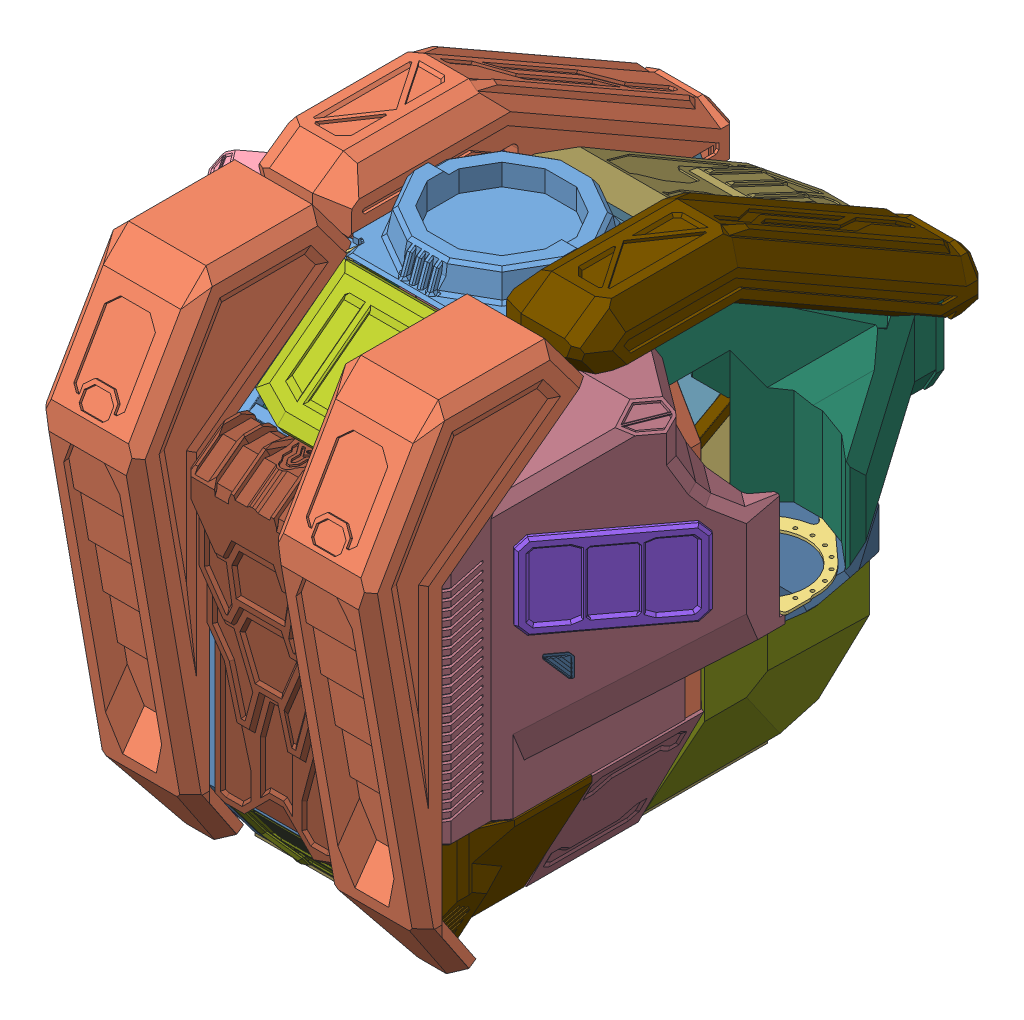
SolidWorks assembly cockpite superficie, configuration Défaut. Lengths in mm. (continued)
Mates (geometry in assembly coordinates): (continued)
- Coaxiale6: concentric anti-aligned: cylinder of axeO20.25_700-1 through (100 1702.1061 -146.8375) axis (-1 0 0) radius 10; cylinder of Capot-1/Capot1-1 through (-490 1702.1061 -146.8375) axis (1 0 0) radius 10
- Distance5: distance = 10 mm anti-aligned: plane of Capot-1/Capot1-1 through (-490 1702.1061 -146.8375) normal (-1 0 0); plane of cockpit_segmentLAT_0-2 through (-500 0 0) normal (1 0 0)
- Coïncidente146: coincident anti-aligned: plane of bras_fixation_1-2 through (-1040 990 -47.0887) normal (0 -1 0); plane of deco_torse2LEFT-1 through (-931.6884 990 -630) normal (0 1 0)
- Coïncidente147: coincident anti-aligned: plane of cockpit_segmentLAT_0-2 through (-500 0 -740) normal (0 0 -1); plane of deco_torse2LEFT-1 through (-173.0822 150 -740) normal (0 0 1)
- Coïncidente148: coincident anti-aligned: plane of cockpit_segmentLAT_0-1 through (80 0 -740) normal (0 0 -1); plane of deco_torse2RIGHT-1 through (336.2329 150 -740) normal (0 0 1)
- Coïncidente149: coincident anti-aligned: plane of bras_fixation_1-1 through (540 990 -47.0887) normal (0 -1 0); plane of deco_torse2RIGHT-1 through (431.6884 990 -630) normal (0 1 0)
- Coïncidente150: coincident anti-aligned: plane of cockpit_segment_40x40_0-3 through (338 1000 -10) normal (0.942847 0 -0.333225); plane of deco_torse2RIGHT-1 through (336.2329 1000 -15) normal (-0.942847 0 0.333225)
- Coïncidente152: coincident anti-aligned: plane of cockpit_segment_40x40_0-4 through (-838 960 -10) normal (-0.942847 0 -0.333225); plane of deco_torse2LEFT-1 through (-836.2329 1000 -15) normal (0.942847 0 0.333225)
- Coïncidente153: coincident anti-aligned: plane of bras_fixation_1-1 through (540 1000 -47.0887) normal (0 1 0); plane of deco_torse1-1 through (277.9178 1000 -180) normal (0 -1 0)
- Coïncidente156: coincident anti-aligned: plane of cockpit_segmentLAT_0-1 through (80 0 -740) normal (0 0 -1); plane of deco_torse1-1 through (277.9178 1000 -740) normal (0 0 1)
- Coïncidente157: coincident anti-aligned: plane of cockpit_segment_40x40_0-1 through (338 1323.2129 -10) normal (0.942847 0 -0.333225); plane of deco_torse1-1 through (277.9178 1350 -180) normal (-0.942847 0 0.333225)
- Coïncidente166: coincident anti-aligned: plane of cockpit_segmentFACE_0-2 through (-593.1411 1740 413.3333) normal (0 1 0); plane of deco_headcollar-1 through (-540 1740 423.19) normal (0 -1 0)
- Coïncidente171: coincident anti-aligned: plane of cockpit_segmentLAT_0-1 through (80 1312 984) normal (0 0.8 0.6); plane of deco_torse4_back-1/deco_torse4_back-1 through (370 1630 560) normal (0 -0.8 -0.6)
- Coïncidente172: coincident anti-aligned: plane of cockpit_segmentLAT_0-2 through (-500 1312 984) normal (0 0.8 0.6); plane of deco_torse4_back-2/deco_torse4_back-1 through (-500 1630 560) normal (0 -0.8 -0.6)
- Coïncidente174: coincident anti-aligned: plane of cockpit_segmentLAT_0-1 through (80 0 960) normal (0 0 1); plane of deco_torse4_back-1/deco_torse4_back-1 through (370 250 960) normal (0 0 -1)
- Coïncidente175: coincident anti-aligned: plane of cockpit_segmentLAT_0-2 through (-500 0 960) normal (0 0 1); plane of deco_torse4_back-2/deco_torse4_back-1 through (-500 250 960) normal (0 0 -1)
- Coïncidente176: coincident aligned: plane of cockpit_segmentLAT_0-1 through (0 0 0) normal (-1 0 0); plane of attache_porte2-2 through (0 1717.0991 489.9076) normal (-1 0 0)
- Coïncidente177: coincident anti-aligned: plane of cockpit_segmentLAT_0-1 through (80 1312 984) normal (0 0.8 0.6); plane of attache_porte2-2 through (10 1737 417.3333) normal (0 -0.8 -0.6)
- Coïncidente180: coincident anti-aligned: plane of cockpit_segmentLAT_0-2 through (-500 1312 984) normal (0 0.8 0.6); plane of attache_porte2-4 through (-500 1737 417.3333) normal (0 -0.8 -0.6)
- Coïncidente181: coincident aligned: plane of cockpit_segmentLAT_0-2 through (-500 0 0) normal (1 0 0); plane of attache_porte2-4 through (-500 1717.0991 489.9076) normal (1 0 0)
- Coaxiale7: concentric aligned: cylinder of attache_porte2-2 through (10 1717.0991 489.9076) axis (-1 0 0) radius 23.5; cylinder of attache_porte2-4 through (-500 1717.0991 489.9076) axis (-1 0 0) radius 23.5
- Coïncidente182: coincident anti-aligned: plane of cockpit_segment_40x40_2_back-2 through (-840 1310.6802 413.3333) normal (-0.902861 0 0.429934); plane of deco_torse5_back-1 through (-674.9206 450 760) normal (0.902861 0 -0.429934)
- Coïncidente186: coincident aligned: plane of cockpit_segmentLAT_0-2 through (-500 0 0) normal (1 0 0); plane of deco_torse4_back-2/deco_torse4_back-1 through (-500 250 960) normal (1 0 0)
- Coïncidente189: coincident anti-aligned: plane of deco_torse4_back-2/deco_torse4_back-1 through (-500 250 960) normal (0 0 -1); plane of deco_torse5_back-1 through (-824.9206 450 960) normal (0 0 1)
- Coïncidente191: coincident anti-aligned: plane of cockpit_segmentLAT_0-2 through (-500 0 -740) normal (0 0 -1); plane of deco_torse1_sym-1 through (-238.4658 1000 -740) normal (0 0 1)
- Coïncidente194: coincident aligned: plane of deco_torse1-1 through (277.9178 1000 -180) normal (0 -1 0); plane of deco_torse1_sym-1 through (-777.9178 1000 -180) normal (0 -1 0)
- Coïncidente195: coincident anti-aligned: plane of cockpit_segment_40x40_0-2 through (-838 1283.2129 -10) normal (-0.942847 0 -0.333225); plane of deco_torse1_sym-1 through (-777.9178 1350 -180) normal (0.942847 0 0.333225)
- Coïncidente197: coincident: plane of deco_headcollar-1 through (-540 1740 423.19) normal (0 -1 0); line of attache_porte2-4 through (-500 1740 413.3333) axis (-1 0 0)
- Coaxiale8: concentric anti-aligned: cylinder of attache_porte2-2 through (10 1717.0991 489.9076) axis (-1 0 0) radius 23.5; cylinder of axeO20_520-1 through (-510 1717.0991 489.9076) axis (1 0 0) radius 10
- Coïncidente198: coincident aligned: plane of attache_porte2-4 through (-510 1717.0991 489.9076) normal (-1 0 0); plane of axeO20_520-1 through (-510 1717.0991 489.9076) normal (-1 0 0)
- Coaxiale9: concentric anti-aligned: cylinder of axeO20_520-1 through (-510 1717.0991 489.9076) axis (1 0 0) radius 10; cylinder of écoutille1-1 through (-5 1717.0991 489.9076) axis (-1 0 0) radius 10
- Distance8: distance = 5 mm anti-aligned: plane of écoutille1-1 through (-495 1761.0064 498.4018) normal (-1 0 0); plane of cockpit_segmentLAT_0-2 through (-500 0 0) normal (1 0 0)
- Coïncidente200: coincident anti-aligned: plane of deco_torse5_back-1 through (-1147.1119 1368.7153 314.3167) normal (0 -1 0); plane of back_trap-1 through (-1155.1093 1368.7153 320.3201) normal (0 1 0)
- Coïncidente201: coincident anti-aligned: plane of deco_torse5_back-1 through (-1165.1221 1098.7153 290.3244) normal (0.600343 0 0.799743); plane of back_trap-1 through (-1173.1196 1098.7153 296.3278) normal (-0.600343 0 -0.799743)
- Coïncidente202: coincident anti-aligned: plane of deco_torse5_back-1 through (-1234.9206 450 214) normal (-0.799743 0 0.600343); plane of back_trap-1 through (-1173.1196 1068.7153 296.3278) normal (0.799743 0 -0.600343)
- Coïncidente203: coincident anti-aligned: plane of bras_fixation_1-2 through (-1040 990 -47.0887) normal (0 -1 0); plane of deco_torse6_airvent-1 through (-834.9206 990 -640.6226) normal (0 1 0)
- Coïncidente204: coincident aligned: plane of deco_torse5_back-1 through (-1234.9206 450 69) normal (-1 0 0); plane of deco_torse6_airvent-1 through (-1234.9206 958 -640.6226) normal (-1 0 0)
- Coïncidente205: coincident anti-aligned: plane of deco_torse5_back-1 through (-1234.9206 450 214) normal (-0.799743 0 0.600343); plane of airvent-1 through (-958.7971 986.7153 581.836) normal (0.799743 0 -0.600343)
- Coïncidente206: coincident anti-aligned: plane of deco_torse5_back-1 through (-945.997 968.7153 582.2305) normal (0.600343 0 0.799743); plane of airvent-1 through (-949.9957 909.7153 585.2322) normal (-0.600343 0 -0.799743)
- Coïncidente207: coincident anti-aligned: plane of deco_torse5_back-1 through (-939.9935 978.7153 590.2279) normal (0 -1 0); plane of airvent-1 through (-943.8039 978.7153 593.4805) normal (0 1 0)
- Coïncidente208: coincident anti-aligned: plane of cockpit_poutre40x80x500-6 through (-500 1328 960) normal (0 0 1); plane of deco_torse7_dos-1 through (-500 230 960) normal (0 0 -1)
- Coïncidente211: coincident anti-aligned: plane of deco_torse4_back-1/deco_torse4_back-1 through (0 250 960) normal (-1 0 0); plane of deco_torse7_dos-1 through (0 230 960) normal (1 0 0)
- Coïncidente212: coincident anti-aligned: plane of cockpit_segmentLAT_0-1 through (80 1312 984) normal (0 0.8 0.6); plane of deco_torse7_dos-1 through (-500 1330 960) normal (0 -0.8 -0.6)
- Coïncidente213: coincident anti-aligned: plane of cockpit_segmentLAT_0-1 through (80 -40 0) normal (0 -1 0); plane of plancher-1 through (-580 -40 740.5405) normal (0 1 0)
- Coïncidente214: coincident: plane of cockpit_segmentLAT_0-1 through (80 0 0) normal (1 0 0); line of plancher-1 through (80 -40 740.5405) axis (0 0 -1)
- Coïncidente216: coincident: line of cockpit_segmentLAT_0-1 through (78 -40 740.5405) axis (-1 0 0); plane of plancher-1 through (-580 -40 740.5405) normal (0 0 1)
- Coïncidente219: coincident anti-aligned: plane of cockpit_segmentFACE_0-1 through (-840 440.3702 69.3774) normal (-0.890435 -0.455111 0); plane of deco_torse8_lateralinferieur-1 through (-599.1619 -30.8347 -6.6667) normal (0.890435 0.455111 0)
- Coïncidente220: coincident aligned: plane of cockpit_segmentFACE_0-2 through (-250 0 413.3333) normal (0 0 1); plane of deco_torse8_lateralinferieur-1 through (-608.0663 -35.3858 413.3333) normal (0 0 1)
- Coïncidente221: coincident: plane of deco_torse5_back-1 through (-674.9206 450 214) normal (0 -1 0); line of deco_torse8_lateralinferieur-1 through (-844.9219 450 413.3333) axis (0 0 -1)
- Coïncidente224: coincident anti-aligned: plane of cockpit_segmentFACE_0-1 through (340 440.3702 69.3774) normal (0.890435 -0.455111 0); plane of deco_torse8_lateralinferieur-2 through (99.1619 -30.8347 413.3333) normal (-0.890435 0.455111 0)
- Coïncidente225: coincident aligned: plane of cockpit_segmentFACE_0-2 through (-250 0 413.3333) normal (0 0 1); plane of deco_torse8_lateralinferieur-2 through (108.0663 -35.3858 413.3333) normal (0 0 1)
- Coïncidente226: coincident aligned: plane of cockpit_segmentLAT_0-1 through (0 0 0) normal (-1 0 0); plane of attache_porte-5 through (0 32.3991 -638.0132) normal (-1 0 0)
- Coïncidente227: coincident anti-aligned: plane of cockpit_segmentLAT_0-1 through (80 -278.2843 -278.2843) normal (0 -0.707107 -0.707107); plane of attache_porte-5 through (10 -33.8763 -522.6923) normal (0 0.707107 0.707107)
- Coïncidente228: coincident anti-aligned: plane of cockpit_segmentLAT_0-2 through (-500 -278.2843 -278.2843) normal (0 -0.707107 -0.707107); plane of attache_porte-6 through (-500 -33.8763 -522.6923) normal (0 0.707107 0.707107)
- Coïncidente229: coincident aligned: plane of cockpit_segmentLAT_0-2 through (-500 0 0) normal (1 0 0); plane of attache_porte-6 through (-500 32.3991 -638.0132) normal (1 0 0)
- Coïncidente230: coincident aligned: line of attache_porte-5 through (10 -40 -516.5685) axis (-1 0 0); line of attache_porte-6 through (-500 -40 -516.5685) axis (-1 0 0)
- Coïncidente232: coincident: plane of plancher-1 through (-580 -40 740.5405) normal (0 1 0); line of attache_porte-5 through (10 -40 -516.5685) axis (-1 0 0)
- Coïncidente233: coincident aligned: plane of attache_porte-5 through (10 32.3991 -638.0132) normal (1 0 0); plane of axeO20_520-2 through (10 32.3991 -638.0132) normal (1 0 0)
- Coaxiale10: concentric anti-aligned: cylinder of attache_porte-6 through (-500 32.3991 -638.0132) axis (-1 0 0) radius 23.5; cylinder of axeO20_520-2 through (-510 32.3991 -638.0132) axis (1 0 0) radius 10
- Coïncidente237: coincident anti-aligned: plane of cockpit_segmentLAT_0-1 through (80 -59.667 129.9889) normal (0 0.417168 -0.90883); plane of internalpanel1_back-1 through (-580 1402.9178 801.3393) normal (0 -0.417168 0.90883)
- Coïncidente238: coincident aligned: plane of cockpit_segmentLAT_0-2 through (-580 0 0) normal (-1 0 0); plane of internalpanel1_back-1 through (-580 1407.0895 792.251) normal (-1 0 0)
- Coïncidente239: coincident aligned: line of cockpit_segmentLAT_0-2 through (-502 485 380) axis (-1 0 0); line of internalpanel1_back-1 through (80 485 380) axis (-1 0 0)
- Coïncidente240: coincident anti-aligned: plane of cockpit_segmentFACE_0-1 through (-800 1300 69.3774) normal (1 0 0); plane of internalpanel2_side-2 through (-800 450 413.3774) normal (-1 0 0)
- Coïncidente241: coincident anti-aligned: line of cockpit_segmentFACE_0-2 through (-800 1300 411.3333) axis (0 0 -1); line of internalpanel2_side-2 through (-800 1300 -10.6226) axis (0 0 1)
- Coïncidente242: coincident anti-aligned: plane of cockpit_segmentFACE_0-1 through (300 1300 69.3774) normal (-1 0 0); plane of internalpanel2_side-1 through (300 450 -10.6226) normal (1 0 0)
- Coïncidente243: coincident aligned: line of cockpit_segmentFACE_0-1 through (300 1300 67.3774) axis (0 0 -1); line of internalpanel2_side-1 through (300 1300 413.3774) axis (0 0 -1)
- Coïncidente244: coincident aligned: plane of cockpit_segmentFACE_0-1 through (-250 0 -10.6226) normal (0 0 -1); plane of internalpanel2_side-1 through (290 450 -10.6226) normal (0 0 -1)
- Coïncidente245: coincident aligned: plane of cockpit_segmentFACE_0-1 through (-250 0 -10.6226) normal (0 0 -1); plane of internalpanel2_side-2 through (-790 450 -10.6226) normal (0 0 -1)
- Coïncidente246: coincident anti-aligned: plane of cockpit_segmentFACE_0-2 through (-570 1700 413.3333) normal (0.866906 -0.498471 0); plane of internalpanel3_upside-1 through (-799.2967 1301.2231 413.3774) normal (-0.866906 0.498471 0)
- Coïncidente247: coincident anti-aligned: plane of cockpit_segmentFACE_0-1 through (70 1700 69.3774) normal (-0.866906 -0.498471 0); plane of internalpanel3_upside-2 through (299.2967 1301.2231 -10.6226) normal (0.866906 0.498471 0)
- Coïncidente248: coincident aligned: plane of cockpit_segmentFACE_0-1 through (-250 0 -10.6226) normal (0 0 -1); plane of internalpanel3_upside-2 through (290.6277 1296.2384 -10.6226) normal (0 0 -1)
- Coïncidente249: coincident aligned: plane of cockpit_segmentFACE_0-1 through (-250 0 -10.6226) normal (0 0 -1); plane of internalpanel3_upside-1 through (-790.6277 1296.2384 -10.6226) normal (0 0 -1)
- Coïncidente250: coincident anti-aligned: line of cockpit_segmentFACE_0-1 through (-570 1700 67.3774) axis (0 0 -1); line of internalpanel3_upside-1 through (-570 1700 -10.6226) axis (0 0 1)
- Coïncidente251: coincident aligned: line of cockpit_segmentFACE_0-2 through (70 1700 411.3333) axis (0 0 -1); line of internalpanel3_upside-2 through (70 1700 413.3774) axis (0 0 -1)
- Coïncidente252: coincident anti-aligned: plane of cockpit_segmentFACE_0-1 through (-800 450 69.3774) normal (0.890435 0.455111 0); plane of internalpanel4_downside-2 through (-570 0 413.3333) normal (-0.890435 -0.455111 0)
- Coïncidente253: coincident aligned: plane of cockpit_segmentFACE_0-2 through (-250 0 413.3333) normal (0 0 1); plane of internalpanel4_downside-2 through (-561.0957 4.5511 413.3333) normal (0 0 1)
- Coïncidente254: coincident anti-aligned: plane of cockpit_segmentFACE_0-1 through (300 450 69.3774) normal (-0.890435 0.455111 0); plane of internalpanel4_downside-1 through (70 0 -10.6226) normal (0.890435 -0.455111 0)
- Coïncidente255: coincident aligned: plane of cockpit_segmentFACE_0-1 through (-250 0 -10.6226) normal (0 0 -1); plane of internalpanel4_downside-1 through (61.0957 4.5511 -10.6226) normal (0 0 -1)
- Coïncidente256: coincident anti-aligned: line of cockpit_segmentFACE_0-1 through (70 0 67.3774) axis (0 0 -1); line of internalpanel4_downside-1 through (70 0 -10.6226) axis (0 0 1)
- Coïncidente257: coincident aligned: line of cockpit_segmentFACE_0-1 through (-570 0 67.3774) axis (0 0 -1); line of internalpanel4_downside-2 through (-570 0 413.3333) axis (0 0 -1)
- Coïncidente258: coincident anti-aligned: plane of cockpit_segmentLAT_0-1 through (80 0 380) normal (0 0 -1); plane of internalpanel5_downback-1 through (80 0 380) normal (0 0 1)
- Coïncidente259: coincident anti-aligned: plane of cockpit_segmentFACE_0-2 through (70 0 413.3333) normal (0 1 0); plane of internalpanel5_downback-1 through (80 0 370) normal (0 -1 0)
- Coïncidente260: coincident aligned: plane of cockpit_segmentLAT_0-1 through (80 0 0) normal (1 0 0); plane of internalpanel5_downback-1 through (80 0 370) normal (1 0 0)
- Coïncidente261: coincident aligned: line of cockpit_segmentLAT_0-2 through (-502 0 -500) axis (-1 0 0); line of internalpanel6_floor-1 through (80 0 -500) axis (-1 0 0)
- Coïncidente262: coincident aligned: plane of cockpit_segmentLAT_0-1 through (80 0 0) normal (1 0 0); plane of internalpanel6_floor-1 through (80 10 -500) normal (1 0 0)
- Coïncidente263: coincident anti-aligned: plane of cockpit_segmentLAT_0-1 through (80 0 0) normal (0 1 0); plane of internalpanel6_floor-1 through (80 0 -500) normal (0 -1 0)
- Distance10: distance = 110 mm anti-aligned: plane of sparco style race seat 1-1 through (-452.7692 280 260) normal (0 0 1); plane of internalpanel5_downback-1 through (80 0 370) normal (0 0 -1)
- Distance11: distance = 270 mm anti-aligned: plane of sparco style race seat 1-1 through (-33.6692 280 -76.55) normal (0 -1 0); plane of internalpanel6_floor-1 through (80 10 -500) normal (0 1 0)
- Coïncidente275: coincident anti-aligned: line of internalpanel2_side-1 through (300 1300 -10.6226) axis (0 -1 0); line of internalpanel7_frontLEFT-2 through (300 450 -10.6226) axis (0 1 0)
- Coïncidente277: coincident: line of internalpanel2_side-1 through (290 1300 -10.6226) axis (1 0 0); plane of internalpanel7_frontLEFT-2 through (4.4348 1300 -700) normal (0 1 0)
- Coïncidente278: coincident: plane of cockpit_segmentLAT_0-1 through (80 0 -700) normal (0 0 1); line of internalpanel7_frontLEFT-2 through (4.4348 1300 -700) axis (0 -1 0)
- Coïncidente279: coincident: line of internalpanel2_side-2 through (-790 1300 -10.6226) axis (-1 0 0); plane of internalpanel8_frontRIGHT-1 through (-1077.08 1300 686.3901) normal (0 1 0)
- Coïncidente280: coincident aligned: line of internalpanel2_side-2 through (-800 450 -10.6226) axis (0 1 0); line of internalpanel8_frontRIGHT-1 through (-800 450 -10.6226) axis (0 1 0)
- Coïncidente282: coincident: plane of cockpit_segmentLAT_0-2 through (-500 0 -700) normal (0 0 1); line of internalpanel8_frontRIGHT-1 through (-504.4348 1300 -700) axis (0 -1 0)
- Coïncidente283: coincident aligned: line of internalpanel3_upside-2 through (61.3309 1695.0153 -10.6226) axis (0.498471 -0.866906 0); line of internalpanel9_frontLup-1 through (59.5239 1698.158 -10.6226) axis (0.498471 -0.866906 0)
- Coïncidente285: coincident: line of internalpanel7_frontLEFT-2 through (290.7574 1300 -6.8049) axis (-0.381763 0 -0.92426); point of internalpanel9_frontLup-1
- Coïncidente286: coincident anti-aligned: line of internalpanel3_upside-1 through (-790.6277 1296.2384 -10.6226) axis (0.498471 0.866906 0); line of internalpanel9_frontLup-2 through (-559.5239 1698.158 -10.6226) axis (-0.498471 -0.866906 0)
- Coïncidente287: coincident: line of internalpanel8_frontRIGHT-1 through (-504.4348 1300 -700) axis (-0.381763 0 0.92426); point of internalpanel9_frontLup-2
- Coïncidente291: coincident aligned: plane of internalpanel2_side-2 through (-790 1300 413.3774) normal (0 1 0); plane of internalpanel10_backsideLEFT-1 through (-790 1300 380) normal (0 1 0)
- Coïncidente296: coincident anti-aligned: line of internalpanel1_back-1 through (-580 485 380) axis (0 0.90883 0.417168); line of internalpanel10_backsideLEFT-1 through (-580 1300 754.0984) axis (0 -0.90883 -0.417168)
- Coïncidente297: coincident anti-aligned: line of internalpanel10_backsideLEFT-1 through (-580 527.1417 380) axis (-0.277211 0.960809 0); line of internalpanel10.5_backsideLEFT-1 through (-790 1254.9989 380) axis (0.277211 -0.960809 0)
- Coïncidente298: coincident anti-aligned: plane of internalpanel10_backsideLEFT-1 through (-790 485 380) normal (0 0 -1); plane of internalpanel10.5_backsideLEFT-1 through (-580 485 380) normal (0 0 1)
- Coïncidente299: coincident: point of internalpanel10_backsideLEFT-1; line of internalpanel10.5_backsideLEFT-1 through (-790 1254.9989 370) axis (0 0 1)
- Coïncidente300: coincident anti-aligned: line of internalpanel1_back-1 through (80 1407.0895 792.251) axis (0 -0.90883 -0.417168); line of internalpanel10_backsideRIGHT-1 through (80 527.1417 388.3406) axis (0 0.90883 0.417168)
- Coïncidente301: coincident aligned: plane of internalpanel10_backsideLEFT-1 through (-790 1300 380) normal (0 1 0); plane of internalpanel10_backsideRIGHT-1 through (290 1300 388.3406) normal (0 1 0)
- Coïncidente303: coincident anti-aligned: plane of internalpanel10_backsideRIGHT-1 through (290 485 388.3406) normal (0 0 -1); plane of internalpanel10.5_backsideRIGHT-1 through (80 485 388.3406) normal (0 0 1)
- Coïncidente304: coincident: point of internalpanel10_backsideRIGHT-1; line of internalpanel10.5_backsideRIGHT-1 through (290 1254.9989 378.3406) axis (0 0 1)
- Parallèle7: parallel anti-aligned: plane of cockpit_segmentLAT_0-1 through (80 0 0) normal (1 0 0); plane of internalpanel10.5_backsideRIGHT-1 through (80 35 388.3406) normal (-1 0 0)
- Coïncidente307: coincident anti-aligned: plane of cockpit_segment_40x40_1_soutien_bras-1 through (-840 990 -10.6226) normal (0 0 -1); plane of deco_torse6_airvent-1 through (-834.9206 990 -10.6226) normal (0 0 1)
- Coïncidente308: coincident anti-aligned: plane of cockpit_segment_40x40_1_soutien_bras-2 through (340 990 -10.6226) normal (0 0 -1); plane of deco_torse6_airventRIGHT-1 through (334.9136 990 -10.6226) normal (0 0 1)
- Coïncidente309: coincident anti-aligned: plane of bras_fixation_1-1 through (540 990 -47.0887) normal (0 -1 0); plane of deco_torse6_airventRIGHT-1 through (334.9136 990 -640.6226) normal (0 1 0)
- Coïncidente310: coincident anti-aligned: plane of deco_torse2RIGHT-1 through (431.6884 1000 -15) normal (0.942847 0 -0.333225); plane of deco_torse6_airventRIGHT-1 through (348.4136 608 -250.6226) normal (-0.942847 0 0.333225)
- Coïncidente312: coincident anti-aligned: plane of cockpit_segmentLAT_0-2 through (-580 0 0) normal (-1 0 0); plane of internalpanel11_backsideUPLEFT-1 through (-580 1310.6802 413.3774) normal (1 0 0)
- Coïncidente314: coincident anti-aligned: plane of internalpanel3_upside-1 through (-790.6277 1296.2384 413.3774) normal (0 0 1); plane of internalpanel11_backsideUPLEFT-1 through (-580 1610.6802 413.3774) normal (0 0 -1)
- Coïncidente318: coincident anti-aligned: plane of cockpit_segment_40x40_2_back-2 through (-580 1310.6802 413.3333) normal (0 1 0); plane of internalpanel11_backsideUPLEFT-1 through (-580 1310.6802 813.3774) normal (0 -1 0)
- Coïncidente319: coincident anti-aligned: plane of cockpit_segmentFACE_0-2 through (-250 0 413.3333) normal (0 0 1); plane of internalpanel11_backsideUPRIGHT-1 through (80 1612.1 413.3333) normal (0 0 -1)
- Coïncidente320: coincident anti-aligned: plane of cockpit_segmentLAT_0-1 through (80 0 0) normal (1 0 0); plane of internalpanel11_backsideUPRIGHT-1 through (80 1677.3174 413.3333) normal (-1 0 0)
- Coïncidente321: coincident anti-aligned: plane of cockpit_segmentLAT_0-1 through (80 1280 960) normal (0 -0.8 -0.6); plane of internalpanel11_backsideUPRIGHT-1 through (80 1690 413.3333) normal (0 0.8 0.6)
- Coïncidente322: coincident aligned: plane of deco_torse5_back-1 through (-674.9206 1740 214) normal (0 1 0); plane of deco_torse5_backRIGHT-1 through (174 1740 214) normal (0 1 0)
- Coïncidente323: coincident anti-aligned: plane of cockpit_segmentLAT_0-1 through (80 0 0) normal (1 0 0); plane of deco_torse5_backRIGHT-1 through (80 1000 214) normal (-1 0 0)
- Coïncidente324: coincident aligned: plane of deco_torse5_back-1 through (-824.9206 450 960) normal (0 0 1); plane of deco_torse5_backRIGHT-1 through (324 450 960) normal (0 0 1)
- Coïncidente325: coincident anti-aligned: plane of deco_torse5_backRIGHT-1 through (646.1912 1368.7153 314.3167) normal (0 -1 0); plane of back_trap-2 through (384.0343 1368.7153 680.2043) normal (0 1 0)
- Coïncidente326: coincident anti-aligned: plane of deco_torse5_backRIGHT-1 through (664.2015 1098.7153 290.3244) normal (-0.600343 0 0.799743); plane of back_trap-2 through (672.1989 1098.7153 296.3278) normal (0.600343 0 -0.799743)
- Coïncidente327: coincident anti-aligned: plane of deco_torse5_backRIGHT-1 through (734 450 214) normal (0.799743 0 0.600343); plane of back_trap-2 through (366.024 1068.7153 704.1966) normal (-0.799743 0 -0.600343)
- Coïncidente328: coincident anti-aligned: plane of deco_torse5_backRIGHT-1 through (439.0729 978.7153 590.2279) normal (0 -1 0); plane of airvent-2 through (407.6514 978.7153 640.4144) normal (0 1 0)
- Coïncidente329: coincident anti-aligned: plane of deco_torse5_backRIGHT-1 through (734 450 214) normal (0.799743 0 0.600343); plane of airvent-2 through (457.8765 986.7153 581.836) normal (-0.799743 0 -0.600343)
- Coïncidente330: coincident anti-aligned: plane of deco_torse5_backRIGHT-1 through (445.0763 968.7153 582.2305) normal (-0.600343 0 0.799743); plane of airvent-2 through (449.075 968.4016 585.2322) normal (0.600343 0 -0.799743)
- Coïncidente332: coincident aligned: plane of deco_torse1_sym-1 through (-777.9178 1350 -180) normal (0 1 0); plane of front_trapLEFT-1 through (-608.1918 1350 -960) normal (0 1 0)
- Coïncidente334: coincident aligned: line of deco_torse1_sym-1 through (-819.9178 1300 -910) axis (0 -1 0); line of front_trapLEFT-1 through (-819.9178 1300 -910) axis (0 -1 0)
- Coïncidente336: coincident aligned: plane of deco_torse1-1 through (277.9178 1350 -180) normal (0 1 0); plane of front_trapRIGHT-1 through (108.1918 1350 -960) normal (0 1 0)
- Coïncidente338: coincident aligned: line of deco_torse1-1 through (319.9178 1300 -910) axis (0 -1 0); line of front_trapRIGHT-1 through (319.9178 1300 -910) axis (0 -1 0)
- Coïncidente343: coincident: plane of cockpit_poutre40x80x500-5 through (0 250 922) normal (0 -1 0); line of deco_torse9_backbas-1 through (-110 250 958.9927) axis (-1 0 0)
- Parallèle9: parallel aligned: plane of cockpit_segmentLAT_0-1 through (80 -370.9057 490.1254) normal (0 -0.603443 0.797406); plane of deco_torse9_backbas-1 through (-500 -44.7272 729.6857) normal (0 -0.603443 0.797406)
- Coïncidente344: coincident anti-aligned: plane of cockpit_segmentLAT_0-1 through (0 0 0) normal (-1 0 0); plane of deco_torse9_backbas-1 through (0 -47.7444 733.6727) normal (1 0 0)
- Coïncidente345: coincident: line of deco_torse7_dos-1 through (-110 230 960) axis (1 0 0); plane of deco_torse9_backbas-1 through (-451.7567 -45.3016 973.865) normal (0 0.050299 0.998734)
- Coïncidente346: coincident: line of deco_torse8_lateralinferieur-2 through (344.9219 450 -6.6667) axis (0 0 1); plane of deco_torse5_backRIGHT-1 through (174 450 214) normal (0 -1 0)
- Coïncidente347: coincident anti-aligned: plane of cockpit_segmentLAT_0-2 through (-580 0 0) normal (-1 0 0); plane of deco_torse10_backbassideLEFT-1 through (-580 -40 963.3333) normal (1 0 0)
- Coïncidente348: coincident anti-aligned: plane of deco_torse5_back-1 through (-674.9206 450 214) normal (0 -1 0); plane of deco_torse10_backbassideLEFT-1 through (-855 450 963.3333) normal (0 1 0)
- Coïncidente349: coincident anti-aligned: plane of cockpit_segmentFACE_0-2 through (-250 0 413.3333) normal (0 0 1); plane of deco_torse10_backbassideLEFT-1 through (-855 -40 413.3333) normal (0 0 -1)
- Coïncidente350: coincident anti-aligned: plane of cockpit_segmentLAT_0-1 through (80 0 0) normal (1 0 0); plane of deco_torse10_backbassideRIGHT-1 through (80 -40 943.3333) normal (-1 0 0)
- Coïncidente351: coincident anti-aligned: plane of deco_torse5_backRIGHT-1 through (174 450 214) normal (0 -1 0); plane of deco_torse10_backbassideRIGHT-1 through (-195 450 963.3333) normal (0 1 0)
- Coïncidente352: coincident anti-aligned: plane of cockpit_segmentFACE_0-2 through (-250 0 413.3333) normal (0 0 1); plane of deco_torse10_backbassideRIGHT-1 through (-195 -40 413.3333) normal (0 0 -1)
- Coaxiale11: concentric anti-aligned: cylinder of axeO20_520-2 through (-510 32.3991 -638.0132) axis (1 0 0) radius 10; cylinder of écoutille2-1 through (0 32.3991 -638.0132) axis (-1 0 0) radius 10
- Coïncidente353: coincident anti-aligned: plane of attache_porte-5 through (0 32.3991 -638.0132) normal (-1 0 0); plane of écoutille2-1 through (0 549.3297 -926.0153) normal (1 0 0)
- Coïncidente358: coincident anti-aligned: plane of attache_porte-4 through (10 1702.1061 -146.8375) normal (1 0 0); plane of deco_headcollar-1 through (10 1760 -106.81) normal (-1 0 0)
- Coïncidente366: coincident anti-aligned: plane of deco_torse1-1 through (360 1350 -740) normal (0 0.868243 -0.496139); plane of deco_torse3_upRIGHT-1 through (390.1918 1340 -757.5) normal (0 -0.868243 0.496139)
- Coïncidente367: coincident anti-aligned: plane of deco_torse1_sym-1 through (-860 1350 -740) normal (0 0.868243 -0.496139); plane of deco_torse3_upLEFT-1 through (-190.1918 1340 -757.5) normal (0 -0.868243 0.496139)
- Coïncidente371: coincident anti-aligned: plane of front_trapLEFT-1 through (-508.1918 1176.7949 -960) normal (0.866025 0.5 0); plane of deco_torse3_upLEFT-1 through (-508.1918 1176.7949 -1026.7218) normal (-0.866025 -0.5 0)
- Coïncidente372: coincident anti-aligned: plane of deco_torse3_upRIGHT-1 through (8.1918 1176.7949 -1026.7218) normal (0.866025 -0.5 0); plane of front_trapRIGHT-1 through (8.1918 1176.7949 -960) normal (-0.866025 0.5 0)
- Coïncidente376: coincident anti-aligned: plane of cockpit_segmentLAT_0-2 through (-500 1740 0) normal (0 1 0); plane of deco_torse3_upLEFT-1 through (-190.1918 1740 642.5) normal (0 -1 0)
- Coïncidente377: coincident anti-aligned: plane of bras_fixation_1-2 through (-1040 990 -47.0887) normal (0 -1 0); plane of deco_torse5_back-1 through (-674.9206 990 214) normal (0 1 0)
- Coïncidente378: coincident anti-aligned: plane of cockpit_segmentLAT_0-2 through (-500 0 0) normal (1 0 0); plane of deco_torse7_dos-1 through (-500 230 960) normal (-1 0 0)
- Coïncidente379: coincident anti-aligned: plane of cockpit_segmentFACE_0-2 through (-250 0 333.3333) normal (0 0 -1); plane of attache_verin_cokpitepaul-2 through (-840 1200.6802 333.3333) normal (0 0 1)
- Coïncidente380: coincident anti-aligned: plane of cockpit_segmentFACE_0-2 through (-840 1310.6802 413.3333) normal (-1 0 0); plane of attache_verin_cokpitepaul-2 through (-840 1200.6802 333.3333) normal (1 0 0)
- Coïncidente381: coincident anti-aligned: plane of cockpit_segmentFACE_0-2 through (-250 0 333.3333) normal (0 0 -1); plane of attache_verin_cokpitepaul-1 through (-840 1270.6802 333.3333) normal (0 0 1)
- Coïncidente382: coincident anti-aligned: plane of cockpit_segmentFACE_0-2 through (-840 1310.6802 413.3333) normal (-1 0 0); plane of attache_verin_cokpitepaul-1 through (-840 1270.6802 333.3333) normal (1 0 0)
- Coïncidente383: coincident anti-aligned: plane of cockpit_segmentFACE_0-2 through (340 1310.6802 413.3333) normal (1 0 0); plane of attache_verin_cokpitepaul-3 through (340 1260.6802 333.3333) normal (-1 0 0)
- Coïncidente384: coincident anti-aligned: plane of cockpit_segmentFACE_0-2 through (-250 0 333.3333) normal (0 0 -1); plane of attache_verin_cokpitepaul-3 through (340 1260.6802 333.3333) normal (0 0 1)
- Coïncidente386: coincident anti-aligned: plane of cockpit_segmentFACE_0-2 through (-250 0 333.3333) normal (0 0 -1); plane of attache_verin_cokpitepaul-4 through (340 1200.6802 333.3333) normal (0 0 1)
- Coïncidente387: coincident anti-aligned: plane of cockpit_segmentFACE_0-2 through (340 1310.6802 413.3333) normal (1 0 0); plane of attache_verin_cokpitepaul-4 through (340 1200.6802 333.3333) normal (-1 0 0)
- Coïncidente389: coincident anti-aligned: plane of cockpit_poutre40x40x366-1 through (-838 1270.6802 333.3333) normal (0 -1 0); plane of attache_verin_cokpitepaul-1 through (-867.2236 1270.6802 306.1097) normal (0 1 0)
- Distance13: distance = 60 mm anti-aligned: plane of attache_verin_cokpitepaul-1 through (-867.2236 1260.6802 306.1097) normal (0 -1 0); plane of attache_verin_cokpitepaul-2 through (-867.2236 1200.6802 306.1097) normal (0 1 0)
- Coïncidente388: coincident anti-aligned: plane of cockpit_poutre40x40x366-3 through (302 1270.6802 333.3774) normal (0 -1 0); plane of attache_verin_cokpitepaul-3 through (367.2236 1270.6802 306.1097) normal (0 1 0)
- Distance16: distance = 60 mm anti-aligned: plane of attache_verin_cokpitepaul-4 through (367.2236 1200.6802 306.1097) normal (0 1 0); plane of attache_verin_cokpitepaul-3 through (367.2236 1260.6802 306.1097) normal (0 -1 0)
